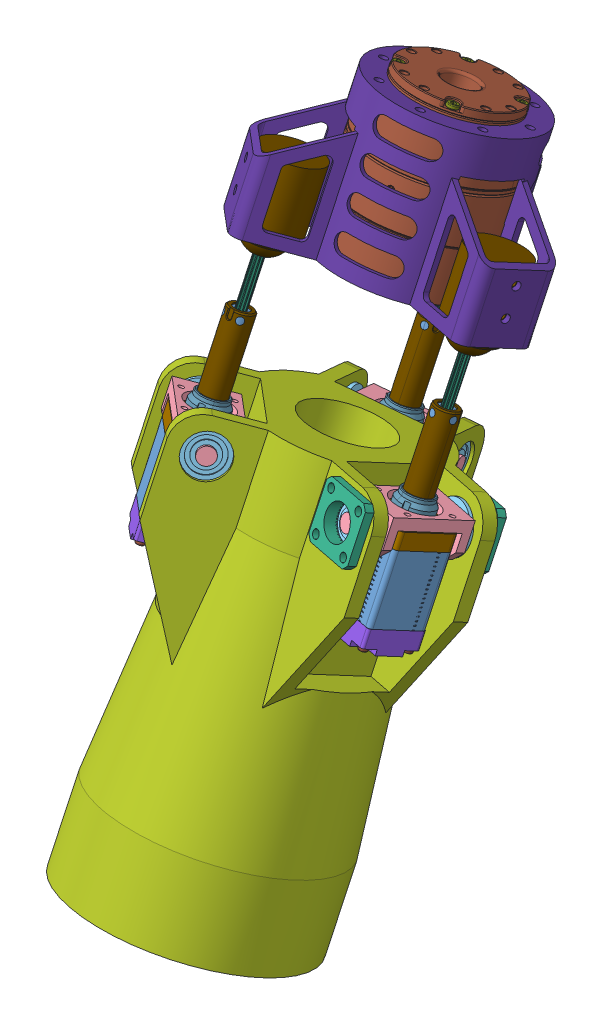
SolidWorks assembly 机械臂总装, configuration 默认. Lengths in mm.
Overall size (122.17 276.98 210.32).
175 component instances, 61 part files, 56 mates.
Components (placement in the parent):
- CRA-RI40-52-PRO-XX 2023.5.4 - Drum-1: CRA-RI40-52-PRO-XX 2023.5.4 - Drum [默认] at (-65.3352 0.778 -52.4868) x (-0.773511 0.267701 0.574471) z (-0.632199 -0.261859 -0.729215) size (67.95 60.31 67.96)
  - CRA-RI40-52-PRO-XX 2023.5.4 - Drum.stp-1: CRA-RI40-52-PRO-XX 2023.5.4 - Drum.stp [默认] at origin size (67.95 60.31 67.96)
    - CRA-RI40-52-PRO-XX_1_ASM.stp-1: CRA-RI40-52-PRO-XX_1_ASM.stp [默认] at origin size (67.95 60.31 67.96)
      - XB11-52__10001_ASM.stp-1: XB11-52__10001_ASM.stp [默认] at (0 16.8 0) x (0.703875 0 -0.710324) z (-0.710324 0 -0.703875) size (66.32 0.8 66.32)
        - XB11-52-06__10001.stp-1: XB11-52-06__10001.stp [默认] at (0 15.8 0) x (0.791272 0 -0.611464) z (-0.611464 0 -0.791272) size (47.28 0.81 47.28)
      - TINYMBS20WITHCONNECTOR2_ASM.stp-1: TINYMBS20WITHCONNECTOR2_ASM.stp [默认] at (2.7275 -27.9719 -6.5848) x (0 -1 0) z (0.92388 0 0.382683) size (0.82 3.25 5.53)
        - FH34SRJ8S05SH_STEP_STEP_ASM.stp-1: FH34SRJ8S05SH_STEP_STEP_ASM.stp [默认] at (-6.4719 -22.2833 0) x (0 0 -1) z (1 0 0) size (5.53 3.25 0.82)
          - NONE-51348.stp-1: NONE-51348.stp [默认] at origin size (0.15 0.3 0.08)
          - NONE-53783.stp-1: NONE-53783.stp [默认] at origin size (0.15 0.3 0.08)
          - NONE-55744.stp-1: NONE-55744.stp [默认] at origin size (0.15 0.08 0.08)
          - NONE-57763.stp-1: NONE-57763.stp [默认] at origin size (0.15 0.08 0.08)
          - NONE-60582.stp-1: NONE-60582.stp [默认] at origin size (0.15 0.3 0.08)
          - NONE-60979.stp-1: NONE-60979.stp [默认] at origin size (0.15 0.3 0.08)
          - NONE-62950.stp-1: NONE-62950.stp [默认] at origin size (0.15 0.3 0.08)
          - NONE-64179.stp-1: NONE-64179.stp [默认] at origin size (0.15 0.3 0.08)
          - NONE-65774.stp-1: NONE-65774.stp [默认] at origin size (0.15 0.08 0.08)
          - NONE-66548.stp-1: NONE-66548.stp [默认] at origin size (0.15 0.35 0.23)
          - NONE-67775.stp-1: NONE-67775.stp [默认] at origin size (0.15 0.35 0.23)
          - NONE-133224.stp-1: NONE-133224.stp [默认] at origin size (0.15 0.08 0.08)
          - NONE-134873.stp-1: NONE-134873.stp [默认] at origin size (0.15 0.3 0.08)
          - NONE-136443.stp-1: NONE-136443.stp [默认] at origin size (0.15 0.08 0.08)
          - NONE-141250.stp-1: NONE-141250.stp [默认] at origin size (0.15 0.35 0.23)
          - NONE-145287.stp-1: NONE-145287.stp [默认] at origin size (0.15 0.08 0.08)
          - NONE-147294.stp-1: NONE-147294.stp [默认] at origin size (0.15 0.08 0.08)
          - NONE-214429.stp-1: NONE-214429.stp [默认] at origin size (0.15 0.9 0.82)
          - NONE-214822.stp-1: NONE-214822.stp [默认] at origin size (0.15 0.3 0.08)
          - NONE-215190.stp-1: NONE-215190.stp [默认] at origin size (0.15 0.08 0.08)
          - NONE-216041.stp-1: NONE-216041.stp [默认] at origin size (0.15 0.35 0.23)
          - NONE-217624.stp-1: NONE-217624.stp [默认] at origin size (0.15 0.35 0.23)
          - NONE-222885.stp-1: NONE-222885.stp [默认] at origin size (0.15 0.35 0.23)
          - NONE-224875.stp-1: NONE-224875.stp [默认] at origin size (0.15 0.35 0.23)
          - NONE-228113.stp-1: NONE-228113.stp [默认] at origin size (0.15 0.9 0.82)
          - NONE-228916.stp-1: NONE-228916.stp [默认] at origin size (0.15 0.35 0.23)
      - CROSS_RECESSED_COUNTERSUNK_HE_1.stp-1: CROSS_RECESSED_COUNTERSUNK_HE_1.stp [默认] at (-21.8123 -33.1 2.8703) x (0 1 0) z (0.6 0 0.8) size (4 3.5 3.5)
      - RI40-52-D12-02__1000.stp-1: RI40-52-D12-02__1000.stp [默认] at (0 -15 0) x (0.382683 0 -0.92388) z (0.92388 0 0.382683) size (52.01 56.6 52)
      - CROSS_RECESSED_CHEESE_HEAD_SC_1.stp-1: CROSS_RECESSED_CHEESE_HEAD_SC_1.stp [默认] at (3.9505 15.5 -22.4044) x (0 -1 0) z (1 0 0) size (5.7 2.98 2.98)
      - MC50-D25X12_5_000.stp-1: MC50-D25X12_5_000.stp [默认] at (0.0001 -26.6014 0.0001) x (0.382686 0 -0.923879) z (0 -1 0) size (48.11 50.01 13.43)
      - CROSS_RECESSED_CHEESE_HEAD_SC_1.stp-2: CROSS_RECESSED_CHEESE_HEAD_SC_1.stp [默认] at (-3.9505 15.5 22.4044) x (0 -1 0) z (-1 0 0) size (5.7 2.98 2.98)
      - CROSS_RECESSED_COUNTERSUNK_HE_1.stp-2: CROSS_RECESSED_COUNTERSUNK_HE_1.stp [默认] at (-3.0048 -33.1 22.5417) x (0 1 0) z (0.395734 0 0.918365) size (4 3.5 3.5)
      - CROSS_RECESSED_CHEESE_HEAD_SC_1.stp-3: CROSS_RECESSED_CHEESE_HEAD_SC_1.stp [默认] at (-18.6357 15.5 13.0489) x (0 -1 0) z (-0.707107 0 -0.707107) size (5.7 2.98 2.98)
      - CROSS_RECESSED_COUNTERSUNK_HE_1.stp-3: CROSS_RECESSED_COUNTERSUNK_HE_1.stp [默认] at (18.8645 -33.1 -12.4259) x (0 1 0) z (0.188455 0 0.982082) size (4 3.5 3.5)
      - _M2X3_M2X3_100.stp-1: _M2X3_M2X3_100.stp [默认] at (-21.8118 -29.6014 2.8705) x (0.8 0 -0.6) z (0.6 0 0.8) size (3.23 5.8 2.8)
      - _M2X3_M2X3_100.stp-2: _M2X3_M2X3_100.stp [默认] at (-13.393 -29.6014 -17.4539) x (0.918365 0 -0.395734) z (0.395734 0 0.918365) size (3.23 5.8 2.8)
      - CROSS_RECESSED_CHEESE_HEAD_SC_1.stp-4: CROSS_RECESSED_CHEESE_HEAD_SC_1.stp [默认] at (-22.4044 15.5 -3.9505) x (0 -1 0) z (0 0 -1) size (5.7 2.98 2.98)
      - CROSS_RECESSED_CHEESE_HEAD_SC_1.stp-5: CROSS_RECESSED_CHEESE_HEAD_SC_1.stp [默认] at (13.0489 15.5 18.6357) x (0 -1 0) z (-0.707107 0 0.707107) size (5.7 2.98 2.98)
      - HEXAGON_SOCKET_HEAD_CAP_SCREW_1.stp-1: HEXAGON_SOCKET_HEAD_CAP_SCREW_1.stp [默认] at (19.8197 15.9 12.6265) x (0 -1 0) z (-0.954517 0 0.298155) size (22.5 4.5 4.5)
      - M2-3_10001.stp-1: M2-3_10001.stp [默认] at (0.7742 21 -17.7331) x (0.020141 0 0.999797) z (-0.999797 0 0.020141) size (4 5.4 4)
      - HEXAGON_SOCKET_HEAD_CAP_SCREW_1.stp-2: HEXAGON_SOCKET_HEAD_CAP_SCREW_1.stp [默认] at (-19.8197 15.9 -12.6265) x (0 -1 0) z (0.954517 0 -0.298155) size (22.5 4.5 4.5)
      - CROSS_RECESSED_CHEESE_HEAD_SC_1.stp-6: CROSS_RECESSED_CHEESE_HEAD_SC_1.stp [默认] at (18.6357 15.5 -13.0489) x (0 -1 0) z (0.707107 0 0.707107) size (5.7 2.98 2.98)
      - M2-3_10001.stp-2: M2-3_10001.stp [默认] at (-17.7331 21 -0.7742) x (0.999797 0 -0.020141) z (0.020141 0 0.999797) size (4 5.4 4)
      - _M2X3_M2X3_100.stp-3: _M2X3_M2X3_100.stp [默认] at (-3.0038 -29.6014 22.5414) x (0.982082 0 -0.188455) z (0.188455 0 0.982082) size (3.23 5.8 2.8)
      - M2-3_10001.stp-3: M2-3_10001.stp [默认] at (-0.7742 21 17.7331) x (-0.020141 0 -0.999797) z (0.999797 0 -0.020141) size (4 5.4 4)
      - _M2X3_M2X3_100.stp-4: _M2X3_M2X3_100.stp [默认] at (18.8646 -29.6014 -12.4267) size (3.23 5.8 2.8)
      - CROSS_RECESSED_COUNTERSUNK_HE_1.stp-4: CROSS_RECESSED_COUNTERSUNK_HE_1.stp [默认] at (-13.393 -33.1 -17.4539) x (0 1 0) z (0 0 1) size (4 3.5 3.5)
      - M2-3_10001.stp-4: M2-3_10001.stp [默认] at (17.7331 21 0.7742) x (-0.999797 0 0.020141) z (-0.020141 0 -0.999797) size (4 5.4 4)
      - CROSS_RECESSED_CHEESE_HEAD_SC_1.stp-7: CROSS_RECESSED_CHEESE_HEAD_SC_1.stp [默认] at (22.4044 15.5 3.9505) x (0 -1 0) z (0 0 1) size (5.7 2.98 2.98)
      - CROSS_RECESSED_CHEESE_HEAD_SC_1.stp-8: CROSS_RECESSED_CHEESE_HEAD_SC_1.stp [默认] at (-13.0489 15.5 -18.6357) x (0 -1 0) z (0.707107 0 -0.707107) size (5.7 2.98 2.98)
- 手腕电机座-1: 手腕电机座 [默认] at (-66.8577 -30.748 -39.8459) x (-0.288066 -0.344371 -0.893547) z (0.956563 -0.147114 -0.251684) size (84.79 53 96.67)
- 球铰2-1: 球铰2 [默认] at (-91.8577 2.9201 -23.4423) x (-0.727754 -0.224677 -0.647992) z (-0.684375 0.29959 0.664738) size (21 30.5 20.4)
- 球铰2-2: 球铰2 [默认] at (-28.733 -6.7882 -40.0512) x (-0.228809 0.371791 0.899677) z (0.972441 0.044781 0.228809) size (21 30.5 20.4)
- 球铰2-3: 球铰2 [默认] at (-76.7583 -21.6149 -82.813) x (0.956563 -0.147114 -0.251684) z (-0.288066 -0.344371 -0.893547) size (21 30.5 20.4)
- 20NC38..31-1: 20NC38..31 [默认] at (-34.2487 -117.8316 4.4347) x (0.046372 0.927308 -0.371416) z (0.972366 0.043263 0.229417) size (109.8 25.88 45.74)
  - 20NC38..31.STEP-1: 20NC38..31.STEP [默认] at origin size (109.8 25.88 45.74)
    - 02-20-38.15________.STEP-1: 02-20-38.15________.STEP [默认] at origin size (39.65 25.88 45.74)
      - 02-20-38.STEP-1: 02-20-38.STEP [默认] at (20.075 0 0) x (0 0 1) z (-1 0 0) size (26.04 25.88 31.46)
        - 02-20-24.15_10-20-001-2.STEP-1: 02-20-24.15_10-20-001-2.STEP [默认] at origin size (20 20 24.15)
        - 13-20-8.5____.STEP-1: 13-20-8.5____.STEP [默认] at (0 0 16.075) x (0 1 0) z (0 0 -1) size (18.2 22.2 10.51)
        - 13-20-12.5______.STEP-1: 13-20-12.5______.STEP [默认] at (0 0 -14.575) x (0.707107 0.707107 0) z (0 0 1) size (18.3 18.3 15.8)
      - 03-20-008______38_______default.STEP-1: 03-20-008______38_______default.STEP [默认] at (3.8 0 0) x (1 0 0) z (0 0.78069 0.624918) size (32.3 16.26 16.27)
        - 06-20-008______38_________01-20-007-1.STEP-1: 06-20-008______38_________01-20-007-1.STEP [默认] at origin size (32.3 7 7)
        - 03-20-4.2-6YK_10-20-006-2.STEP-1: 03-20-4.2-6YK_10-20-006-2.STEP [默认] at (24.2 0 0) x (0 0.91534 0.402682) z (-1 0 0) size (12.06 12.08 4.2)
        - 10-20-001__________.STEP-1: 10-20-001__________.STEP [默认] at (16.9 0 0) x (0 0 1) z (-1 0 0) size (11.2 11.2 1.3)
        - 08-20-001______1_______07-20-001-1.STEP-1: 08-20-001______1_______07-20-001-1.STEP [默认] at (22.1 0 0) x (0 0 1) z (-1 0 0) size (11 11 1)
        - 08-20-001______1_______07-20-001-1.STEP-2: 08-20-001______1_______07-20-001-1.STEP [默认] at (11.4 0 0) x (0 0 1) z (-1 0 0) size (11 11 1)
        - 03-20-4.2-6YK_10-20-006-2.STEP-2: 03-20-4.2-6YK_10-20-006-2.STEP [默认] at (19 0 0) x (0 0.888249 0.459362) z (-1 0 0) size (12.06 12.08 4.2)
        - 03-20-4.2-6YK_10-20-006-2.STEP-3: 03-20-4.2-6YK_10-20-006-2.STEP [默认] at (13.5 0 0) x (0 0.91534 0.402682) z (-1 0 0) size (12.06 12.08 4.2)
        - 03-20-4.2-6YK_10-20-006-2.STEP-4: 03-20-4.2-6YK_10-20-006-2.STEP [默认] at (8.3 0 0) x (0 0.888249 0.459362) z (-1 0 0) size (12.06 12.08 4.2)
      - 01-20-003__20__________________.STEP-1: 01-20-003__20__________________.STEP [默认] at origin size (8.8 20 20)
      - 01-20-001__20__________________.STEP-1: 01-20-001__20__________________.STEP [默认] at (31.35 0 0) x (0 0 1) z (1 0 0) size (20 20 8.3)
      - 09-20-001____9X__5X4)_09-20-001.STEP-1: 09-20-001____9X__5X4)_09-20-001.STEP [默认] at (33.1 0 0) x (1 0 0) z (0 0.994502 0.104719) size (3 9 9)
      - 09-20-001____9X__5X4)_09-20-001.STEP-2: 09-20-001____9X__5X4)_09-20-001.STEP [默认] at (3.8 0 0) x (1 0 0) z (0 -0.49427 -0.869308) size (3 9 9)
      - 11-20-002__M2-37__20-42__.STEP-1: 11-20-002__M2-37__20-42__.STEP [默认] at (0.39 -7.7 7.7) x (0 0 -1) z (1 0 0) size (3 3 33)
      - 11-20-002__M2-37__20-42__.STEP-2: 11-20-002__M2-37__20-42__.STEP [默认] at (0.39 -7.7 -7.7) x (0 1 0) z (1 0 0) size (3 3 33)
      - 11-20-002__M2-37__20-42__.STEP-3: 11-20-002__M2-37__20-42__.STEP [默认] at (0.39 7.7 -7.7) x (0 0 1) z (1 0 0) size (3 3 33)
      - 11-20-002__M2-37__20-42__.STEP-4: 11-20-002__M2-37__20-42__.STEP [默认] at (0.39 7.7 7.7) x (0 -1 0) z (1 0 0) size (3 3 33)
      - 06-20-099__20___________20____________YK.STEP-1: 06-20-099__20___________20____________YK.STEP [默认] at (31.1 0 0) x (0 -0.624918 0.78069) z (-1 0 0) size (6.01 6.01 10)
      - 14-20-001__20-28____________________.STEP-1: 14-20-001__20-28____________________.STEP [默认] at (6.15 0 -8.6) x (0 -1 0) z (0 0 1) size (10.5 3.4 24.5)
    - 07-20-007__________________.STEP-1: 07-20-007__________________.STEP [默认] at (39.65 0 0) x (-1 0 0) z (0 -0.999857 -0.016895) size (6 12.92 13)
    - 07-20-013-2______________.STEP-1: 07-20-013-2______________.STEP [默认] at (68.4 0 0) x (0 -0.714016 0.700129) z (1 0 0) size (3.42 3.5 41.4)
    - 07-20-013-3______________.STEP-1: 07-20-013-3______________.STEP [默认] at (20.15 0 0) x (0 0.924225 0.381849) z (1 0 0) size (8 8 56.63)
    - 07-20-006__20______.STEP-1: 07-20-006__20______.STEP [默认] at (67.9 0 0) x (0 0.924225 0.381849) z (1 0 0) size (4.8 4.8 0.5)
    - 07-20-013-1__20_____________08-20-002-1.STEP-1: 07-20-013-1__20_____________08-20-002-1.STEP [默认] at (36.1 0 0) x (0 0.004204 -0.999991) z (1 0 0) size (9.01 9.01 35.91)
    - 07-20-002__20________________.STEP-1: 07-20-002__20________________.STEP [默认] at (69.65 0 0) x (0 0.004204 -0.999991) z (1 0 0) size (9.01 9.01 3.1)
- 螺纹转换套-1: 螺纹转换套 [默认] at (-30.0844 -34.5593 -28.9185) x (-0.195243 -0.356231 -0.913772) z (0.046372 0.927308 -0.371416) size (5 5 5)
- 球-1: 球 [默认] at (-29.7853 -28.5782 -31.3141) x (-0.55453 -0.285367 -0.781705) z (0.830871 -0.242211 -0.500987) size (14 13.45 14)
- 球-2: 球 [默认] at (-92.91 -18.87 -14.7052) x (0.833324 -0.238487 -0.498693) z (0.551058 0.287142 0.783508) size (14 13.45 14)
- 螺纹转换套-2: 螺纹转换套 [默认] at (-78.0965 -49.3819 -71.6684) x (0.952783 0.073148 0.29471) z (0.044309 0.926671 -0.373253) size (5 5 5)
- 螺纹转换套-3: 螺纹转换套 [默认] at (-93.1916 -24.8538 -12.3142) x (-0.196131 -0.355877 -0.91372) z (0.043661 0.927725 -0.370703) size (5 5 5)
- 球-3: 球 [默认] at (-77.8107 -43.4049 -74.0759) x (0.898492 0.126374 0.420407) z (-0.436749 0.353993 0.827006) size (14 13.45 14)
- 20NC38..31-2: 20NC38..31 [默认] at (-82.0754 -132.597 -38.1503) x (0.044309 0.926671 -0.373253) z (-0.288139 -0.345888 -0.892937) size (109.8 25.88 45.74)
  - 20NC38..31.STEP-1: 20NC38..31.STEP [默认] at origin size (109.8 25.88 45.74)
    - 02-20-38.15________.STEP-1: 02-20-38.15________.STEP [默认] at origin size (39.65 25.88 45.74)
      - 02-20-38.STEP-1: 02-20-38.STEP [默认] at (20.075 0 0) x (0 0 1) z (-1 0 0) size (26.04 25.88 31.46)
        - 02-20-24.15_10-20-001-2.STEP-1: 02-20-24.15_10-20-001-2.STEP [默认] at origin size (20 20 24.15)
        - 13-20-8.5____.STEP-1: 13-20-8.5____.STEP [默认] at (0 0 16.075) x (0 1 0) z (0 0 -1) size (18.2 22.2 10.51)
        - 13-20-12.5______.STEP-1: 13-20-12.5______.STEP [默认] at (0 0 -14.575) x (0.707107 0.707107 0) z (0 0 1) size (18.3 18.3 15.8)
      - 03-20-008______38_______default.STEP-1: 03-20-008______38_______default.STEP [默认] at (3.8 0 0) x (1 0 0) z (0 0.78069 0.624918) size (32.3 16.26 16.27)
        - 06-20-008______38_________01-20-007-1.STEP-1: 06-20-008______38_________01-20-007-1.STEP [默认] at origin size (32.3 7 7)
        - 03-20-4.2-6YK_10-20-006-2.STEP-1: 03-20-4.2-6YK_10-20-006-2.STEP [默认] at (24.2 0 0) x (0 0.91534 0.402682) z (-1 0 0) size (12.06 12.08 4.2)
        - 10-20-001__________.STEP-1: 10-20-001__________.STEP [默认] at (16.9 0 0) x (0 0 1) z (-1 0 0) size (11.2 11.2 1.3)
        - 08-20-001______1_______07-20-001-1.STEP-1: 08-20-001______1_______07-20-001-1.STEP [默认] at (22.1 0 0) x (0 0 1) z (-1 0 0) size (11 11 1)
        - 08-20-001______1_______07-20-001-1.STEP-2: 08-20-001______1_______07-20-001-1.STEP [默认] at (11.4 0 0) x (0 0 1) z (-1 0 0) size (11 11 1)
        - 03-20-4.2-6YK_10-20-006-2.STEP-2: 03-20-4.2-6YK_10-20-006-2.STEP [默认] at (19 0 0) x (0 0.888249 0.459362) z (-1 0 0) size (12.06 12.08 4.2)
        - 03-20-4.2-6YK_10-20-006-2.STEP-3: 03-20-4.2-6YK_10-20-006-2.STEP [默认] at (13.5 0 0) x (0 0.91534 0.402682) z (-1 0 0) size (12.06 12.08 4.2)
        - 03-20-4.2-6YK_10-20-006-2.STEP-4: 03-20-4.2-6YK_10-20-006-2.STEP [默认] at (8.3 0 0) x (0 0.888249 0.459362) z (-1 0 0) size (12.06 12.08 4.2)
      - 01-20-003__20__________________.STEP-1: 01-20-003__20__________________.STEP [默认] at origin size (8.8 20 20)
      - 01-20-001__20__________________.STEP-1: 01-20-001__20__________________.STEP [默认] at (31.35 0 0) x (0 0 1) z (1 0 0) size (20 20 8.3)
      - 09-20-001____9X__5X4)_09-20-001.STEP-1: 09-20-001____9X__5X4)_09-20-001.STEP [默认] at (33.1 0 0) x (1 0 0) z (0 0.994502 0.104719) size (3 9 9)
      - 09-20-001____9X__5X4)_09-20-001.STEP-2: 09-20-001____9X__5X4)_09-20-001.STEP [默认] at (3.8 0 0) x (1 0 0) z (0 -0.49427 -0.869308) size (3 9 9)
      - 11-20-002__M2-37__20-42__.STEP-1: 11-20-002__M2-37__20-42__.STEP [默认] at (0.39 -7.7 7.7) x (0 0 -1) z (1 0 0) size (3 3 33)
      - 11-20-002__M2-37__20-42__.STEP-2: 11-20-002__M2-37__20-42__.STEP [默认] at (0.39 -7.7 -7.7) x (0 1 0) z (1 0 0) size (3 3 33)
      - 11-20-002__M2-37__20-42__.STEP-3: 11-20-002__M2-37__20-42__.STEP [默认] at (0.39 7.7 -7.7) x (0 0 1) z (1 0 0) size (3 3 33)
      - 11-20-002__M2-37__20-42__.STEP-4: 11-20-002__M2-37__20-42__.STEP [默认] at (0.39 7.7 7.7) x (0 -1 0) z (1 0 0) size (3 3 33)
      - 06-20-099__20___________20____________YK.STEP-1: 06-20-099__20___________20____________YK.STEP [默认] at (31.1 0 0) x (0 -0.624918 0.78069) z (-1 0 0) size (6.01 6.01 10)
      - 14-20-001__20-28____________________.STEP-1: 14-20-001__20-28____________________.STEP [默认] at (6.15 0 -8.6) x (0 -1 0) z (0 0 1) size (10.5 3.4 24.5)
    - 07-20-007__________________.STEP-1: 07-20-007__________________.STEP [默认] at (39.65 0 0) x (-1 0 0) z (0 -0.999857 -0.016895) size (6 12.92 13)
    - 07-20-013-2______________.STEP-1: 07-20-013-2______________.STEP [默认] at (68.4 0 0) x (0 -0.714016 0.700129) z (1 0 0) size (3.42 3.5 41.4)
    - 07-20-013-3______________.STEP-1: 07-20-013-3______________.STEP [默认] at (20.15 0 0) x (0 0.924225 0.381849) z (1 0 0) size (8 8 56.63)
    - 07-20-006__20______.STEP-1: 07-20-006__20______.STEP [默认] at (67.9 0 0) x (0 0.924225 0.381849) z (1 0 0) size (4.8 4.8 0.5)
    - 07-20-013-1__20_____________08-20-002-1.STEP-1: 07-20-013-1__20_____________08-20-002-1.STEP [默认] at (36.1 0 0) x (0 0.004204 -0.999991) z (1 0 0) size (9.01 9.01 35.91)
    - 07-20-002__20________________.STEP-1: 07-20-002__20________________.STEP [默认] at (69.65 0 0) x (0 0.004204 -0.999991) z (1 0 0) size (9.01 9.01 3.1)
- 20NC38..31-3: 20NC38..31 [默认] at (-97.1124 -108.1635 20.9749) x (0.043661 0.927725 -0.370703) z (-0.684447 0.298072 0.665346) size (109.8 25.88 45.74)
  - 20NC38..31.STEP-1: 20NC38..31.STEP [默认] at origin size (109.8 25.88 45.74)
    - 02-20-38.15________.STEP-1: 02-20-38.15________.STEP [默认] at origin size (39.65 25.88 45.74)
      - 02-20-38.STEP-1: 02-20-38.STEP [默认] at (20.075 0 0) x (0 0 1) z (-1 0 0) size (26.04 25.88 31.46)
        - 02-20-24.15_10-20-001-2.STEP-1: 02-20-24.15_10-20-001-2.STEP [默认] at origin size (20 20 24.15)
        - 13-20-8.5____.STEP-1: 13-20-8.5____.STEP [默认] at (0 0 16.075) x (0 1 0) z (0 0 -1) size (18.2 22.2 10.51)
        - 13-20-12.5______.STEP-1: 13-20-12.5______.STEP [默认] at (0 0 -14.575) x (0.707107 0.707107 0) z (0 0 1) size (18.3 18.3 15.8)
      - 03-20-008______38_______default.STEP-1: 03-20-008______38_______default.STEP [默认] at (3.8 0 0) x (1 0 0) z (0 0.78069 0.624918) size (32.3 16.26 16.27)
        - 06-20-008______38_________01-20-007-1.STEP-1: 06-20-008______38_________01-20-007-1.STEP [默认] at origin size (32.3 7 7)
        - 03-20-4.2-6YK_10-20-006-2.STEP-1: 03-20-4.2-6YK_10-20-006-2.STEP [默认] at (24.2 0 0) x (0 0.91534 0.402682) z (-1 0 0) size (12.06 12.08 4.2)
        - 10-20-001__________.STEP-1: 10-20-001__________.STEP [默认] at (16.9 0 0) x (0 0 1) z (-1 0 0) size (11.2 11.2 1.3)
        - 08-20-001______1_______07-20-001-1.STEP-1: 08-20-001______1_______07-20-001-1.STEP [默认] at (22.1 0 0) x (0 0 1) z (-1 0 0) size (11 11 1)
        - 08-20-001______1_______07-20-001-1.STEP-2: 08-20-001______1_______07-20-001-1.STEP [默认] at (11.4 0 0) x (0 0 1) z (-1 0 0) size (11 11 1)
        - 03-20-4.2-6YK_10-20-006-2.STEP-2: 03-20-4.2-6YK_10-20-006-2.STEP [默认] at (19 0 0) x (0 0.888249 0.459362) z (-1 0 0) size (12.06 12.08 4.2)
        - 03-20-4.2-6YK_10-20-006-2.STEP-3: 03-20-4.2-6YK_10-20-006-2.STEP [默认] at (13.5 0 0) x (0 0.91534 0.402682) z (-1 0 0) size (12.06 12.08 4.2)
        - 03-20-4.2-6YK_10-20-006-2.STEP-4: 03-20-4.2-6YK_10-20-006-2.STEP [默认] at (8.3 0 0) x (0 0.888249 0.459362) z (-1 0 0) size (12.06 12.08 4.2)
      - 01-20-003__20__________________.STEP-1: 01-20-003__20__________________.STEP [默认] at origin size (8.8 20 20)
      - 01-20-001__20__________________.STEP-1: 01-20-001__20__________________.STEP [默认] at (31.35 0 0) x (0 0 1) z (1 0 0) size (20 20 8.3)
      - 09-20-001____9X__5X4)_09-20-001.STEP-1: 09-20-001____9X__5X4)_09-20-001.STEP [默认] at (33.1 0 0) x (1 0 0) z (0 0.994502 0.104719) size (3 9 9)
      - 09-20-001____9X__5X4)_09-20-001.STEP-2: 09-20-001____9X__5X4)_09-20-001.STEP [默认] at (3.8 0 0) x (1 0 0) z (0 -0.49427 -0.869308) size (3 9 9)
      - 11-20-002__M2-37__20-42__.STEP-1: 11-20-002__M2-37__20-42__.STEP [默认] at (0.39 -7.7 7.7) x (0 0 -1) z (1 0 0) size (3 3 33)
      - 11-20-002__M2-37__20-42__.STEP-2: 11-20-002__M2-37__20-42__.STEP [默认] at (0.39 -7.7 -7.7) x (0 1 0) z (1 0 0) size (3 3 33)
      - 11-20-002__M2-37__20-42__.STEP-3: 11-20-002__M2-37__20-42__.STEP [默认] at (0.39 7.7 -7.7) x (0 0 1) z (1 0 0) size (3 3 33)
      - 11-20-002__M2-37__20-42__.STEP-4: 11-20-002__M2-37__20-42__.STEP [默认] at (0.39 7.7 7.7) x (0 -1 0) z (1 0 0) size (3 3 33)
      - 06-20-099__20___________20____________YK.STEP-1: 06-20-099__20___________20____________YK.STEP [默认] at (31.1 0 0) x (0 -0.624918 0.78069) z (-1 0 0) size (6.01 6.01 10)
      - 14-20-001__20-28____________________.STEP-1: 14-20-001__20-28____________________.STEP [默认] at (6.15 0 -8.6) x (0 -1 0) z (0 0 1) size (10.5 3.4 24.5)
    - 07-20-007__________________.STEP-1: 07-20-007__________________.STEP [默认] at (39.65 0 0) x (-1 0 0) z (0 -0.999857 -0.016895) size (6 12.92 13)
    - 07-20-013-2______________.STEP-1: 07-20-013-2______________.STEP [默认] at (68.4 0 0) x (0 -0.714016 0.700129) z (1 0 0) size (3.42 3.5 41.4)
    - 07-20-013-3______________.STEP-1: 07-20-013-3______________.STEP [默认] at (20.15 0 0) x (0 0.924225 0.381849) z (1 0 0) size (8 8 56.63)
    - 07-20-006__20______.STEP-1: 07-20-006__20______.STEP [默认] at (67.9 0 0) x (0 0.924225 0.381849) z (1 0 0) size (4.8 4.8 0.5)
    - 07-20-013-1__20_____________08-20-002-1.STEP-1: 07-20-013-1__20_____________08-20-002-1.STEP [默认] at (36.1 0 0) x (0 0.004204 -0.999991) z (1 0 0) size (9.01 9.01 35.91)
    - 07-20-002__20________________.STEP-1: 07-20-002__20________________.STEP [默认] at (69.65 0 0) x (0 0.004204 -0.999991) z (1 0 0) size (9.01 9.01 3.1)
- 电缸座-1: 电缸座 [默认] at (-95.2721 -69.0599 5.3498) x (0.727754 0.224677 0.647992) z (-0.043661 -0.927725 0.370703) size (42 20 14)
- F696.ZZ-1: F696.ZZ [默认] at (-84.6614 -72.1838 17.6646) x (0.148454 0.870814 -0.468663) z (0.669578 -0.437269 -0.600384) size (17 5 17)
- F696.ZZ-2: F696.ZZ [默认] at (-106.494 -78.9241 -1.7752) x (-0.284553 0.958575 -0.012786) z (-0.624022 -0.175083 0.761539) size (17 5 17)
- 轴承端盖-2: 轴承端盖 [默认] at (-38.1559 -76.2394 13.1516) x (-0.044781 -0.927236 0.371791) z (0.228809 -0.371791 -0.899677) size (20.14 20.14 5)
- 轴承端盖-3: 轴承端盖 [默认] at (-27.0815 -94.234 -30.3928) x (-0.044781 -0.927236 0.371791) z (-0.228809 0.371791 0.899677) size (20.14 20.14 5)
- 电缸座-4: 电缸座 [默认] at (-32.2941 -78.7455 -11.2205) x (0.228809 -0.371791 -0.899677) z (-0.046372 -0.927308 0.371416) size (42 20 14)
- 电缸座-5: 电缸座 [默认] at (-80.2078 -93.5378 -53.8829) x (-0.956563 0.147114 0.251684) z (-0.044309 -0.926671 0.373253) size (42 20 14)
- 手腕关节-1: 手腕关节 [默认] at (-75.7512 -214.8969 33.9919) x (0.972441 0.044781 0.228809) z (-0.228809 0.371791 0.899677) size (93.36 150 107.8)
- F696.ZZ-7: F696.ZZ [默认] at (-29.1866 -90.8136 -22.1158) x (-0.103795 0.909608 -0.402293) z (-0.967922 -0.18543 -0.169536) size (17 5 17)
- F696.ZZ-9: F696.ZZ [默认] at (-94.8664 -97.8178 -47.4949) x (-0.050847 0.765907 -0.640938) z (0.287058 0.625895 0.725158) size (17 5 17)
- F696.ZZ-10: F696.ZZ [默认] at (-66.1695 -102.2312 -55.0454) x (-0.036507 0.796088 -0.604079) z (-0.289231 -0.587028 -0.756137) size (17 5 17)
- F696.ZZ-11: F696.ZZ [默认] at (-36.0508 -79.6598 4.8745) x (-0.228512 0.877857 -0.42089) z (0.946271 0.30189 0.115903) size (17 5 17)
Mates (geometry in assembly coordinates):
- 重合2: coincident anti-aligned: plane of 手腕电机座-1 through (-91.4115 21.8166 -16.6063) normal (0.684375 -0.29959 -0.664738); plane of 球铰2-1 through (-98.102 -35.0535 2.1363) normal (-0.684375 0.29959 0.664738)
- 同心6: concentric aligned: cylinder of 手腕电机座-1 through (-93.3819 -1.1469 -20.3204) axis (-0.684375 0.29959 0.664738) radius 1.5; cylinder of 球铰2-1 through (-92.0131 -1.7461 -21.6498) axis (-0.684375 0.29959 0.664738) radius 1.25
- 同心7: concentric anti-aligned: cylinder of 20NC38..31-1/20NC38..31.STEP-1/07-20-013-2______________.STEP-1 through (-29.3889 -20.6497 -34.4897) axis (0.046372 0.927308 -0.371416) radius 1.25; cylinder of 螺纹转换套-1 through (-29.8526 -29.9228 -30.7756) axis (-0.046372 -0.927308 0.371416) radius 1.25
- 同心8: concentric aligned: cylinder of 螺纹转换套-1 through (-29.8526 -29.9228 -30.7756) axis (-0.046372 -0.927308 0.371416) radius 2.5; cylinder of 球-1 through (-29.8526 -29.9228 -30.7756) axis (-0.046372 -0.927308 0.371416) radius 2.5
- 重合3: coincident anti-aligned: plane of 螺纹转换套-1 through (-29.8526 -29.9228 -30.7756) normal (0.046372 0.927308 -0.371416); plane of 球-1 through (-29.8526 -29.9228 -30.7756) normal (-0.046372 -0.927308 0.371416)
- 同心10: concentric aligned: cylinder of 手腕电机座-1 through (-93.8297 -10.4192 -16.6024) axis (-0.684375 0.29959 0.664738) radius 1.5; cylinder of 球铰2-1 through (-92.4609 -11.0184 -17.9319) axis (-0.684375 0.29959 0.664738) radius 1.25
- 同心11: concentric anti-aligned: cylinder of 螺纹转换套-2 through (-77.8749 -44.7486 -73.5347) axis (-0.044309 -0.926671 0.373253) radius 2.5; cylinder of 20NC38..31-2/20NC38..31.STEP-1/07-20-013-2______________.STEP-1 through (-77.4318 -35.4819 -77.2672) axis (0.044309 0.926671 -0.373253) radius 1.25
- 同心12: concentric aligned: cylinder of 螺纹转换套-2 through (-77.8749 -44.7486 -73.5347) axis (-0.044309 -0.926671 0.373253) radius 2.5; cylinder of 球-3 through (-77.8749 -44.7486 -73.5347) axis (-0.044309 -0.926671 0.373253) radius 2.5
- 重合4: coincident anti-aligned: plane of 螺纹转换套-2 through (-77.8749 -44.7486 -73.5347) normal (0.044309 0.926671 -0.373253); plane of 球-3 through (-77.8749 -44.7486 -73.5347) normal (-0.044309 -0.926671 0.373253)
- 同心13: concentric anti-aligned: cylinder of 螺纹转换套-3 through (-92.9733 -20.2152 -14.1677) axis (-0.043661 -0.927725 0.370703) radius 2.5; axis of 20NC38..31-3/20NC38..31.STEP-1/07-20-013-2______________.STEP-1 through (-92.5367 -10.9379 -17.8747) axis (0.043661 0.927725 -0.370703)
- 同心14: concentric aligned: cylinder of 球-2 through (-92.9733 -20.2152 -14.1677) axis (-0.043661 -0.927725 0.370703) radius 2.5; cylinder of 螺纹转换套-3 through (-92.9733 -20.2152 -14.1677) axis (-0.043661 -0.927725 0.370703) radius 2.5
- 重合5: coincident anti-aligned: plane of 球-2 through (-92.9733 -20.2152 -14.1677) normal (-0.043661 -0.927725 0.370703); plane of 螺纹转换套-3 through (-92.9733 -20.2152 -14.1677) normal (0.043661 0.927725 -0.370703)
- 重合6: coincident anti-aligned: plane of 20NC38..31-3/20NC38..31.STEP-1/02-20-38.15________.STEP-1/01-20-001__20__________________.STEP-1 through (-95.0786 -68.3274 17.996) normal (0.043661 0.927725 -0.370703); plane of 电缸座-1 through (-95.4467 -72.7708 6.8326) normal (-0.043661 -0.927725 0.370703)
- 同心17: concentric aligned: cylinder of 20NC38..31-3/20NC38..31.STEP-1/02-20-38.15________.STEP-1/01-20-001__20__________________.STEP-1 through (-95.4467 -72.7708 6.8326) axis (0.043661 0.927725 -0.370703) radius 8; cylinder of 电缸座-1 through (-95.4467 -72.7708 6.8326) axis (0.043661 0.927725 -0.370703) radius 8
- 同心18: concentric anti-aligned: cylinder of 20NC38..31-3/20NC38..31.STEP-1/02-20-38.15________.STEP-1/01-20-001__20__________________.STEP-1 through (-84.5073 -71.9443 6.1429) axis (-0.043661 -0.927725 0.370703) radius 0.75; line of 电缸座-1 through (-84.5727 -73.3359 6.699) axis (0.043661 0.927725 -0.370703)
- 同心19: concentric anti-aligned: cylinder of 电缸座-1 through (-80.2948 -70.8357 21.5526) axis (-0.727754 -0.224677 -0.647992) radius 3; cylinder of F696.ZZ-1 through (-79.4147 -70.564 22.3363) axis (0.727754 0.224677 0.647992) radius 3
- 重合7: coincident anti-aligned: plane of 电缸座-1 through (-84.3557 -65.6897 15.0697) normal (0.727754 0.224677 0.647992); plane of F696.ZZ-1 through (-83.9933 -68.2651 15.5556) normal (-0.727754 -0.224677 -0.647992)
- 同心20: concentric anti-aligned: cylinder of F696.ZZ-1 through (-79.4147 -70.564 22.3363) axis (0.727754 0.224677 0.647992) radius 7.5; cylinder of F696.ZZ-2 through (-111.7407 -80.5439 -6.4468) axis (-0.727754 -0.224677 -0.647992) radius 7.5
- 重合8: coincident anti-aligned: plane of 电缸座-1 through (-106.1884 -72.43 -4.3701) normal (-0.727754 -0.224677 -0.647992); plane of F696.ZZ-2 through (-108.9127 -70.7762 -1.8838) normal (0.727754 0.224677 0.647992)
- 同心33: concentric anti-aligned: cylinder of F696.ZZ-6 through (-2.5623 -103.2131 137.2832) axis (-0.228809 0.371791 0.899677) radius 3; cylinder of 电缸座-4 through (-37.4237 -77.4291 10.2726) axis (0.228809 -0.371791 -0.899677) radius 3
- 重合17: coincident anti-aligned: plane of 20NC38..31-1/20NC38..31.STEP-1/02-20-38.15________.STEP-1/01-20-001__20__________________.STEP-1 through (-22.2696 -85.2473 -15.4321) normal (0.046372 0.927308 -0.371416); plane of 电缸座-4 through (-32.4796 -82.4548 -9.7349) normal (-0.046372 -0.927308 0.371416)
- 同心35: concentric anti-aligned: cylinder of 20NC38..31-1/20NC38..31.STEP-1/02-20-38.15________.STEP-1/01-20-001__20__________________.STEP-1 through (-38.1354 -84.2597 -18.986) axis (-0.046372 -0.927308 0.371416) radius 0.75; cylinder of 电缸座-4 through (-38.205 -85.6507 -18.4289) axis (0.046372 0.927308 -0.371416) radius 1
- 同心36: concentric anti-aligned: cylinder of 20NC38..31-1/20NC38..31.STEP-1/02-20-38.15________.STEP-1/01-20-001__20__________________.STEP-1 through (-41.6591 -78.5342 -5.131) axis (-0.046372 -0.927308 0.371416) radius 0.75; cylinder of 电缸座-4 through (-41.7286 -79.9251 -4.5739) axis (0.046372 0.927308 -0.371416) radius 1
- 重合18: coincident anti-aligned: plane of 20NC38..31-2/20NC38..31.STEP-1/02-20-38.15________.STEP-1/01-20-001__20__________________.STEP-1 through (-90.965 -98.934 -57.8405) normal (0.044309 0.926671 -0.373253); plane of 电缸座-5 through (-80.385 -97.2445 -52.3899) normal (-0.044309 -0.926671 0.373253)
- 同心38: concentric aligned: cylinder of 20NC38..31-2/20NC38..31.STEP-1/02-20-38.15________.STEP-1/01-20-001__20__________________.STEP-1 through (-80.385 -97.2445 -52.3899) axis (0.044309 0.926671 -0.373253) radius 8; cylinder of 电缸座-5 through (-80.385 -97.2445 -52.3899) axis (0.044309 0.926671 -0.373253) radius 8
- 距离1: distance = 15 mm anti-aligned: plane of 螺纹转换套-2 through (-78.0965 -49.3819 -71.6684) normal (-0.044309 -0.926671 0.373253); plane of 20NC38..31-2/20NC38..31.STEP-1/07-20-013-2______________.STEP-1 through (-77.4318 -35.4819 -77.2672) normal (0.044309 0.926671 -0.373253)
- 距离2: distance = 15 mm anti-aligned: plane of 螺纹转换套-3 through (-93.1916 -24.8538 -12.3142) normal (-0.043661 -0.927725 0.370703); plane of 20NC38..31-3/20NC38..31.STEP-1/07-20-013-2______________.STEP-1 through (-92.5367 -10.9379 -17.8747) normal (0.043661 0.927725 -0.370703)
- 距离3: distance = 15 mm anti-aligned: plane of 螺纹转换套-1 through (-30.0844 -34.5593 -28.9185) normal (-0.046372 -0.927308 0.371416); plane of 20NC38..31-1/20NC38..31.STEP-1/07-20-013-2______________.STEP-1 through (-29.3889 -20.6497 -34.4897) normal (0.046372 0.927308 -0.371416)
- 重合23: coincident anti-aligned: plane of F696.ZZ-6 through (0.831 -101.9217 129.5992) normal (0.228809 -0.371791 -0.899677); plane of 电缸座-4 through (-35.7262 -73.1687 2.2746) normal (-0.228809 0.371791 0.899677)
- 同心48: concentric: sphere of 球铰2-3; sphere of 球-3
- 同心50: concentric anti-aligned: cylinder of 轴承端盖-5 through (7.4846 -119.5382 97.7789) axis (0.228809 -0.371791 -0.899677) radius 6; cylinder of 电缸座-4 through (-27.8137 -93.0443 -27.5138) axis (-0.228809 0.371791 0.899677) radius 3
- 重合24: coincident anti-aligned: plane of 手腕关节-1 through (-68.2381 -142.1049 -12.1852) normal (-0.228809 0.371791 0.899677); plane of F696.ZZ-7 through (-29.6904 -84.4377 -26.2126) normal (0.228809 -0.371791 -0.899677)
- 同心52: concentric anti-aligned: cylinder of 手腕关节-1 through (-27.173 -94.0853 -30.0329) axis (-0.228809 0.371791 0.899677) radius 7.5; cylinder of F696.ZZ-7 through (-27.537 -93.494 -28.6019) axis (0.228809 -0.371791 -0.899677) radius 7.5
- 同心53: concentric anti-aligned: cylinder of 电缸座-4 through (-27.8137 -93.0443 -27.5138) axis (-0.228809 0.371791 0.899677) radius 3; cylinder of F696.ZZ-7 through (-27.537 -93.494 -28.6019) axis (0.228809 -0.371791 -0.899677) radius 3
- 重合25: coincident anti-aligned: plane of 电缸座-4 through (-28.862 -84.3224 -24.7157) normal (0.228809 -0.371791 -0.899677); plane of F696.ZZ-7 through (-30.0688 -83.0819 -25.5352) normal (-0.228809 0.371791 0.899677)
- 同心54: concentric aligned: cylinder of 手腕关节-1 through (-27.173 -94.0853 -30.0329) axis (-0.228809 0.371791 0.899677) radius 7.5; cylinder of F696.ZZ-11 through (-37.7004 -76.9794 11.3607) axis (-0.228809 0.371791 0.899677) radius 7.5
- 重合26: coincident anti-aligned: plane of 手腕关节-1 through (-75.6515 -130.0588 16.9644) normal (0.228809 -0.371791 -0.899677); plane of F696.ZZ-11 through (-38.0392 -72.6298 2.7975) normal (-0.228809 0.371791 0.899677)
- 重合27: coincident anti-aligned: plane of 轴承端盖-2 through (-37.4694 -77.3547 10.4525) normal (0.228809 -0.371791 -0.899677); plane of 手腕关节-1 through (-80.6019 -207.0149 53.065) normal (-0.228809 0.371791 0.899677)
- 平行1: parallel aligned: plane of 轴承端盖-2 through (-38.4058 -52.4049 45.4758) normal (0.044781 0.927236 -0.371791); plane of 手腕关节-1 through (-69.0341 -75.8115 -21.7768) normal (0.044781 0.927236 -0.371791)
- 同心55: concentric aligned: cylinder of 轴承端盖-2 through (-37.4694 -77.3547 10.4525) axis (-0.228809 0.371791 0.899677) radius 6; cylinder of 手腕关节-1 through (-27.173 -94.0853 -30.0329) axis (-0.228809 0.371791 0.899677) radius 7.5
- 同心56: concentric aligned: circle of 轴承端盖-3; cylinder of 手腕关节-1 through (-27.173 -94.0853 -30.0329) axis (-0.228809 0.371791 0.899677) radius 7.5
- 平行2: parallel aligned: plane of 轴承端盖-3 through (-25.9296 -99.392 -70.2057) normal (0.044781 0.927236 -0.371791); plane of 手腕关节-1 through (-69.0341 -75.8115 -21.7768) normal (0.044781 0.927236 -0.371791)
- 重合30: coincident anti-aligned: plane of 轴承端盖-3 through (-27.7679 -93.1187 -27.6937) normal (-0.228809 0.371791 0.899677); plane of 手腕关节-1 through (-70.9005 -222.7789 14.9187) normal (0.228809 -0.371791 -0.899677)
- 同心57: concentric anti-aligned: cylinder of F696.ZZ-1 through (-79.4147 -70.564 22.3363) axis (0.727754 0.224677 0.647992) radius 7.5; cylinder of 手腕关节-1 through (-78.2571 -70.2066 23.3669) axis (-0.727754 -0.224677 -0.647992) radius 7.5
- 重合32: coincident anti-aligned: plane of F696.ZZ-1 through (-82.6747 -65.3831 14.9272) normal (0.727754 0.224677 0.647992); plane of 手腕关节-1 through (-60.1552 -132.4421 12.8871) normal (-0.727754 -0.224677 -0.647992)
- 同心58: concentric aligned: cylinder of 手腕关节-1 through (-103.2842 -96.5232 -45.28) axis (0.956563 -0.147114 -0.251684) radius 7.5; cylinder of F696.ZZ-10 through (-59.2732 -103.2918 -56.8599) axis (0.956563 -0.147114 -0.251684) radius 7.5
- 重合33: coincident anti-aligned: plane of 手腕关节-1 through (-56.4485 -138.4651 -1.6877) normal (-0.956563 0.147114 0.251684); plane of F696.ZZ-10 through (-65.2954 -96.4371 -59.878) normal (0.956563 -0.147114 -0.251684)
- 同心59: concentric anti-aligned: cylinder of 手腕关节-1 through (-103.2842 -96.5232 -45.28) axis (0.956563 -0.147114 -0.251684) radius 7.5; cylinder of F696.ZZ-9 through (-101.7627 -96.7571 -45.6804) axis (-0.956563 0.147114 0.251684) radius 7.5
- 重合34: coincident anti-aligned: plane of 手腕关节-1 through (-87.4411 -133.6986 6.4669) normal (0.956563 -0.147114 -0.251684); plane of F696.ZZ-9 through (-96.3956 -91.8969 -51.9999) normal (-0.956563 0.147114 0.251684)
- 重合35: coincident anti-aligned: plane of 电缸座-5 through (-65.8594 -95.7445 -57.6582) normal (0.956563 -0.147114 -0.251684); plane of F696.ZZ-10 through (-66.3338 -98.6488 -57.7637) normal (-0.956563 0.147114 0.251684)
- 同心60: concentric anti-aligned: cylinder of 电缸座-5 through (-60.4301 -103.1139 -56.5555) axis (-0.956563 0.147114 0.251684) radius 3; cylinder of F696.ZZ-10 through (-59.2732 -103.2918 -56.8599) axis (0.956563 -0.147114 -0.251684) radius 3
- 同心61: concentric: sphere of 球铰2-1; sphere of 球-2
- 同心63: concentric: sphere of 球铰2-2; sphere of 球-1
- 同心64: concentric anti-aligned: cylinder of 20NC38..31-2/20NC38..31.STEP-1/02-20-38.15________.STEP-1/01-20-001__20__________________.STEP-1 through (-89.9028 -97.385 -57.8874) axis (-0.044309 -0.926671 0.373253) radius 0.75; line of 电缸座-5 through (-89.9692 -98.775 -57.3275) axis (0.044309 0.926671 -0.373253)
- 重合36: coincident anti-aligned: plane of CRA-RI40-52-PRO-XX 2023.5.4 - Drum-1/CRA-RI40-52-PRO-XX 2023.5.4 - Drum.stp-1/CRA-RI40-52-PRO-XX_1_ASM.stp-1/RI40-52-D12-02__1000.stp-1 through (-64.6187 15.6138 -58.4354) normal (0.044781 0.927236 -0.371791); plane of 手腕电机座-1 through (-64.6187 15.6138 -58.4354) normal (-0.044781 -0.927236 0.371791)
- 同心65: concentric aligned: cylinder of CRA-RI40-52-PRO-XX 2023.5.4 - Drum-1/CRA-RI40-52-PRO-XX 2023.5.4 - Drum.stp-1/CRA-RI40-52-PRO-XX_1_ASM.stp-1/RI40-52-D12-02__1000.stp-1 through (-64.9187 9.4013 -55.9444) axis (0.044781 0.927236 -0.371791) radius 20; cylinder of 手腕电机座-1 through (-64.6607 14.7431 -58.0863) axis (0.044781 0.927236 -0.371791) radius 28
